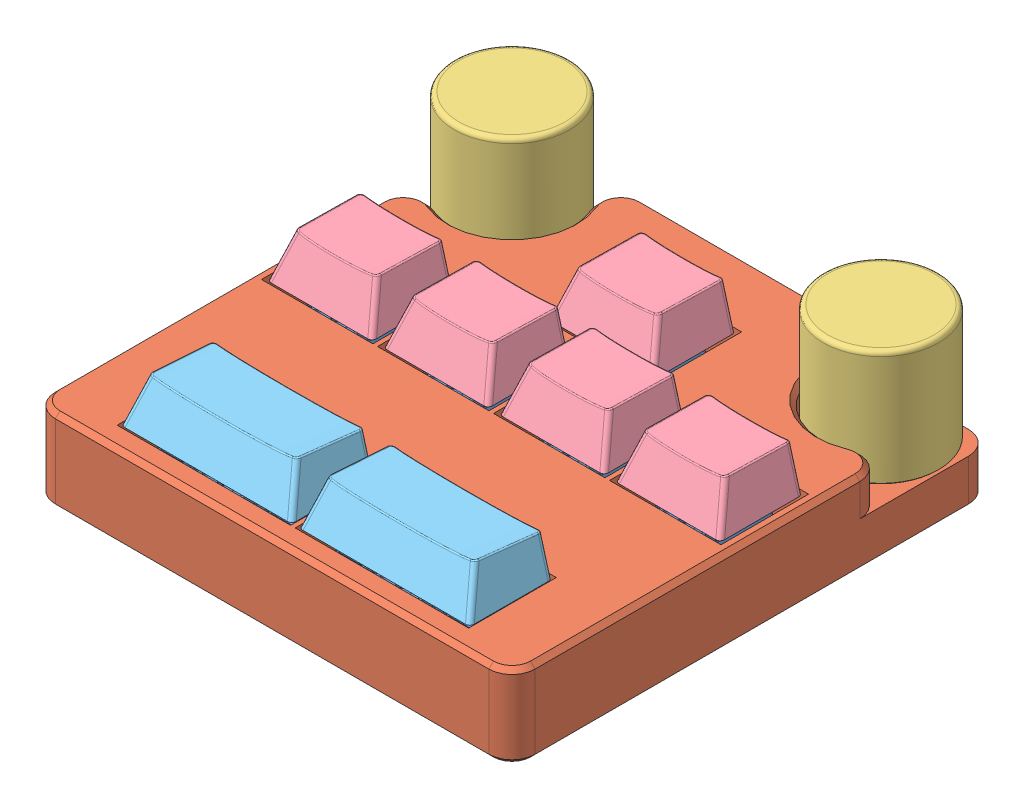
SolidWorks assembly Assembled_v2, configuration Default. Lengths in mm.
Overall size (105.48 36 104.75).
12 component instances, 6 part files, 31 mates.
Components (placement in the parent):
- PCB-1: PCB [Default] at (-1.9549 40.7594 121.5758) x (1 0 0) z (0 1 0) size (100.01 100.01 28.5)
- Case0-1: Case0 [Default] at (98.0451 52.7594 121.5758) x (-1 0 0) z (0 0 1) size (104 18 104)
- Knob-1: Knob [Default] at (88.0406 45.759 31.5758) size (25.49 25 25.49)
- Knob-2: Knob [Default] at (8.0495 45.759 31.5758) size (25.49 25 25.49)
- 1.25xR3-1: 1.25xR3 [Default] at (10.2701 52.5894 66.5258) x (1 0 0) z (0 0 1) size (22.8 11.64 18.12)
- 1.25xR3-2: 1.25xR3 [Default] at (35.4201 52.5894 66.5258) x (1 0 0) z (0 0 1) size (22.8 11.64 18.12)
- 1.25xR3-3: 1.25xR3 [Default] at (60.5701 52.5894 66.5258) x (1 0 0) z (0 0 1) size (22.8 11.64 18.12)
- 1.25xR3-4: 1.25xR3 [Default] at (85.7201 52.5894 66.5258) x (1 0 0) z (0 0 1) size (22.8 11.64 18.12)
- 1.25xR3-5: 1.25xR3 [Default] at (47.9951 52.5894 43.3258) x (1 0 0) z (0 0 1) size (22.8 11.64 18.12)
- 2.00xR2-1: 2.00xR2 [Default] at (67.2951 52.5894 109.5258) x (1 0 0) z (0 0 1) size (37.1 9.19 18.04)
- 2.00xR2-2: 2.00xR2 [Default] at (28.6951 52.5894 109.5258) x (1 0 0) z (0 0 1) size (37.1 9.19 18.04)
- Case1-1: Case1 [Default] at (48.0451 36.7594 71.5758) x (1 0 0) z (0 0 -1) size (100 2 100)
Mates (geometry in assembly coordinates):
- 重合1: coincident anti-aligned: plane of PCB-1 through (1.0451 40.3479 21.5758) normal (0 0 -1); plane of Case0-1 through (95.0451 34.7594 21.5758) normal (0 0 1)
- 重合2: coincident anti-aligned: plane of PCB-1 through (98.0451 40.3479 24.5758) normal (1 0 0); plane of Case0-1 through (98.0451 34.7594 24.5758) normal (-1 0 0)
- 重合3: coincident anti-aligned: plane of PCB-1 through (-1.9549 40.7594 118.5758) normal (0 1 0); plane of Case0-1 through (98.0451 40.7594 121.5758) normal (0 -1 0)
- 同心1: concentric anti-aligned: circle of PCB-1; circle of Knob-1
- 重合5: coincident anti-aligned: plane of PCB-1 through (88.0406 65.759 31.5758) normal (0 1 0); plane of Knob-1 through (88.0406 65.759 31.5758) normal (0 -1 0)
- 重合6: coincident anti-aligned: plane of PCB-1 through (8.0495 65.759 31.5758) normal (0 1 0); plane of Knob-2 through (8.0495 65.759 31.5758) normal (0 -1 0)
- 同心2: concentric anti-aligned: circle of PCB-1; circle of Knob-2
- 重合7: coincident anti-aligned: plane of PCB-1 through (10.8201 56.2894 64.5258) normal (0 0 -1); plane of 1.25xR3-1 through (9.7201 64.1192 64.5258) normal (0 0 1)
- 重合8: coincident anti-aligned: plane of PCB-1 through (12.2701 56.2894 67.1758) normal (1 0 0); plane of 1.25xR3-1 through (12.2701 64.1192 65.9258) normal (-1 0 0)
- 重合9: coincident anti-aligned: plane of PCB-1 through (10.2701 52.5894 66.5258) normal (0 1 0); plane of 1.25xR3-1 through (10.2701 52.5894 66.5258) normal (0 -1 0)
- 重合10: coincident anti-aligned: plane of PCB-1 through (35.9701 56.2894 64.5258) normal (0 0 -1); plane of 1.25xR3-2 through (34.8701 64.1192 64.5258) normal (0 0 1)
- 重合11: coincident anti-aligned: plane of PCB-1 through (33.4201 56.2894 67.1758) normal (-1 0 0); plane of 1.25xR3-2 through (33.4201 64.1192 67.1258) normal (1 0 0)
- 重合12: coincident anti-aligned: plane of PCB-1 through (35.4201 52.5894 66.5258) normal (0 1 0); plane of 1.25xR3-2 through (35.4201 52.5894 66.5258) normal (0 -1 0)
- 重合13: coincident anti-aligned: plane of PCB-1 through (61.1201 56.2894 64.5258) normal (0 0 -1); plane of 1.25xR3-3 through (60.0201 64.1192 64.5258) normal (0 0 1)
- 重合14: coincident anti-aligned: plane of PCB-1 through (62.5701 56.2894 67.1758) normal (1 0 0); plane of 1.25xR3-3 through (62.5701 64.1192 65.9258) normal (-1 0 0)
- 重合15: coincident anti-aligned: plane of PCB-1 through (60.5701 52.5894 66.5258) normal (0 1 0); plane of 1.25xR3-3 through (60.5701 52.5894 66.5258) normal (0 -1 0)
- 重合16: coincident anti-aligned: plane of PCB-1 through (87.7201 56.2894 67.1758) normal (1 0 0); plane of 1.25xR3-4 through (87.7201 64.1192 65.9258) normal (-1 0 0)
- 重合17: coincident anti-aligned: plane of PCB-1 through (86.2701 56.2894 64.5258) normal (0 0 -1); plane of 1.25xR3-4 through (85.1701 64.1192 64.5258) normal (0 0 1)
- 重合18: coincident anti-aligned: plane of PCB-1 through (85.7201 52.5894 66.5258) normal (0 1 0); plane of 1.25xR3-4 through (85.7201 52.5894 66.5258) normal (0 -1 0)
- 重合19: coincident anti-aligned: plane of PCB-1 through (45.9951 56.2894 43.9758) normal (-1 0 0); plane of 1.25xR3-5 through (45.9951 64.1192 43.9258) normal (1 0 0)
- 重合20: coincident anti-aligned: plane of PCB-1 through (48.5451 56.2894 41.3258) normal (0 0 -1); plane of 1.25xR3-5 through (47.4451 64.1192 41.3258) normal (0 0 1)
- 重合21: coincident anti-aligned: plane of PCB-1 through (47.9951 52.5894 43.3258) normal (0 1 0); plane of 1.25xR3-5 through (47.9951 52.5894 43.3258) normal (0 -1 0)
- 重合22: coincident anti-aligned: plane of PCB-1 through (69.2951 56.2894 110.1758) normal (1 0 0); plane of 2.00xR2-1 through (69.2951 52.5894 108.9258) normal (-1 0 0)
- 重合23: coincident anti-aligned: plane of PCB-1 through (67.8451 56.2894 107.5258) normal (0 0 -1); plane of 2.00xR2-1 through (66.7451 52.5894 107.5258) normal (0 0 1)
- 重合24: coincident anti-aligned: plane of PCB-1 through (67.2951 52.5894 109.5258) normal (0 1 0); plane of 2.00xR2-1 through (67.2951 52.5894 109.5258) normal (0 -1 0)
- 重合25: coincident anti-aligned: plane of PCB-1 through (29.2451 56.2894 107.5258) normal (0 0 -1); plane of 2.00xR2-2 through (16.1451 52.5894 107.5258) normal (0 0 1)
- 重合26: coincident anti-aligned: plane of PCB-1 through (26.6951 56.2894 110.1758) normal (-1 0 0); plane of 2.00xR2-2 through (26.6951 52.5894 110.1258) normal (1 0 0)
- 重合27: coincident anti-aligned: plane of PCB-1 through (28.6951 52.5894 109.5258) normal (0 1 0); plane of 2.00xR2-2 through (28.6951 52.5894 109.5258) normal (0 -1 0)
- 重合28: coincident anti-aligned: plane of Case0-1 through (95.0451 34.7594 121.5758) normal (0 0 -1); plane of Case1-1 through (1.0451 34.7594 121.5758) normal (0 0 1)
- 重合29: coincident anti-aligned: plane of Case0-1 through (-1.9549 34.7594 24.5758) normal (1 0 0); plane of Case1-1 through (-1.9549 34.7594 118.5758) normal (-1 0 0)
- 重合30: coincident aligned: plane of Case0-1 through (95.0451 34.7594 118.5758) normal (0 -1 0); plane of Case1-1 through (95.0451 34.7594 118.5758) normal (0 -1 0)
